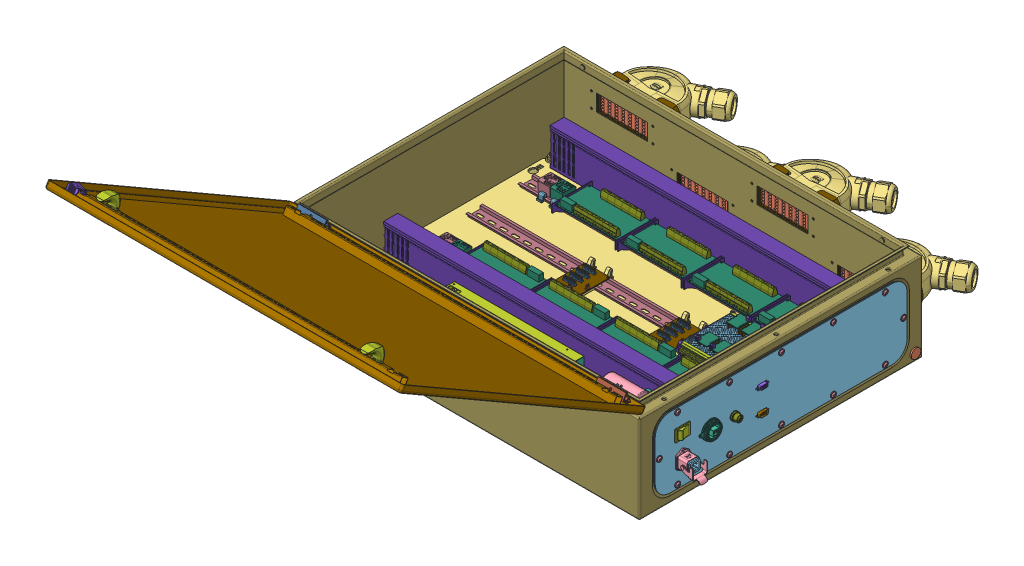
SolidWorks assembly _main_cabinet, configuration Default. Lengths in mm. (continued)
Components (placement in the parent): (continued)
- custom_perfboard-1: custom_perfboard [Default] at (151.5551 53.8 -20.003) size (162 55.7 125.4) (continued)
  - 3857 Adafruit Feather M4 Express headers 2-1: 3857 Adafruit Feather M4 Express headers 2 [Default] at (160.01 12.6 -94.45) x (-1 0 0) z (0 1 0) size (50.85 22.86 20.37) (continued)
    - 3857 Adafruit Feather M4 Express-1: 3857 Adafruit Feather M4 Express [Default] at origin size (50.85 22.86 6.37) (continued)
      - 3857 Adafruit Feather M4 Express(2)^3857 Adafruit Feather M4 Express-1: 3857 Adafruit Feather M4 Express(2)^3857 Adafruit Feather M4 Express [Default] at origin size (50.85 22.86 6.37) (virtual) (continued)
        - PCB Component^3857 Adafruit Feather M4 Express(2)_3857 Adafruit Feather M4 Express-1: PCB Component^3857 Adafruit Feather M4 Express(2)_3857 Adafruit Feather M4 Express [Default] at origin size (50.85 22.86 6.37) (virtual) (continued)
          - MBR120^PCB Component_3857 Adafruit Feather M4 Express(2)_3857 Adafruit Feather M4 Express-1: MBR120^PCB Component_3857 Adafruit Feather M4 Express(2)_3857 Adafruit Feather M4 Express [Default] at (10.35 12.319 1.57) x (-1 0 0) z (0 0 1) size (3.6 1.4 1.35) (virtual)
          - DMG341^PCB Component_3857 Adafruit Feather M4 Express(2)_3857 Adafruit Feather M4 Express-1: DMG341^PCB Component_3857 Adafruit Feather M4 Express(2)_3857 Adafruit Feather M4 Express [Default] at (9.398 9.842 1.57) size (3.04 2.64 1.12) (virtual)
          - 100K^PCB Component_3857 Adafruit Feather M4 Express(2)_3857 Adafruit Feather M4 Express-1: 100K^PCB Component_3857 Adafruit Feather M4 Express(2)_3857 Adafruit Feather M4 Express [Default] at (22.67 17.208 1.57) x (0 1 0) z (0 0 1) size (3.05 1.6 0.5) (virtual)
          - ATSAMD51J^PCB Component_3857 Adafruit Feather M4 Express(2)_3857 Adafruit Feather M4 Express-1: ATSAMD51J^PCB Component_3857 Adafruit Feather M4 Express(2)_3857 Adafruit Feather M4 Express [Default] at (30.162 11.049 1.57) x (0 1 0) z (0 0 1) size (9 9 0.8) (virtual)
          - 10uH^PCB Component_3857 Adafruit Feather M4 Express(2)_3857 Adafruit Feather M4 Express-1: 10uH^PCB Component_3857 Adafruit Feather M4 Express(2)_3857 Adafruit Feather M4 Express [Default] at (21.082 11.811 1.57) x (0 -1 0) z (0 0 1) size (2.7 2 2) (virtual)
    - header_m16-1: header_m16 [Default] at (5.08 1.27 -2.5) x (1 0 0) z (0 -1 0) size (40.64 11.5 2.5)
    - header_m12-1: header_m12 [Default] at (15.24 21.59 -2.5) x (1 0 0) z (0 -1 0) size (30.48 11.5 2.5)
    - header_f12-1: header_f12 [Default] at (15.115 21.59 -11) x (1 0 0) z (0 -1 0) size (30.73 11.5 2.5)
    - header_f16-1: header_f16 [Default] at (4.955 1.27 -11) x (1 0 0) z (0 -1 0) size (40.89 11.5 2.5)
  - dil_socket_2x7_populated-1: dil_socket_2x7_populated [Default] at (124.45 5.35 -38.57) x (0 0 -1) z (1 0 0) size (19.5 11.05 10.16)
    - dil_socket_2x7-1: dil_socket_2x7 [Default] at origin size (17.78 8.25 10.16)
    - dil_package_2x7-1: dil_package_2x7 [Default] at (-0.86 0.5 0) size (19.5 6.8 8.17)
  - header_m4-1: header_m4 [Default] at (8.88 4.1 -15.71) x (0 0 1) z (1 0 0) size (10.16 11.5 2.5)
  - header_m4-2: header_m4 [Default] at (6.34 4.1 -15.71) x (0 0 1) z (1 0 0) size (10.16 11.5 2.5)
  - screw_terminal_4x_2.54pitch_Multicomp_MP008515-1: screw_terminal_4x_2.54pitch_Multicomp_MP008515 [Default] at (153.05 1.6 -12.93) size (6.3 12.4 10.64)
  - screw_terminal_4x_2.54pitch_Multicomp_MP008515-2: screw_terminal_4x_2.54pitch_Multicomp_MP008515 [Default] at (153.05 1.6 -30.71) size (6.3 12.4 10.64)
  - 4-20mA_R_click_in_headers-6: 4-20mA_R_click_in_headers [Default] at (78.75 12.6 -33.49) x (-1 0 0) z (0 0 -1) size (25.4 24.5 30.48)
    - 4-20mA_R_click-1: 4-20mA_R_click [Default] at origin size (25.4 1.7 30.48)
    - header_m8-1: header_m8 [Default] at (1.25 -2.5 -22.86) x (0 0 1) z (-1 0 0) size (20.32 11.5 2.5)
    - header_m8-2: header_m8 [Default] at (24.15 -2.5 -2.54) x (0 0 -1) z (1 0 0) size (20.32 11.5 2.5)
    - screw_terminal_2x_2.54pitch-1: screw_terminal_2x_2.54pitch [Default] at (24.765 1.7 -23.545) x (0 0 -1) z (1 0 0) size (6.3 12.6 5.6)
    - header_f8-1: header_f8 [Default] at (24.15 -11 -2.415) x (0 0 -1) z (1 0 0) size (20.57 11.5 2.5)
    - header_f8-2: header_f8 [Default] at (1.25 -11 -22.985) x (0 0 1) z (-1 0 0) size (20.57 11.5 2.5)
  - Damen_CNC_2340-1_DIN-Rail_Mount_for_Eurocard_PCB_100x160mm_STEP214-1: Damen_CNC_2340-1_DIN-Rail_Mount_for_Eurocard_PCB_100x160mm_STEP214 [Default] at (158 -16.0731 10.0976) x (0 1 0) z (-1 0 0) size (37.6 125.4 162)
    - 2340-1_DIN-Rail_Mount_for_Eurocard_PCB_100x160mm_STEP214^Damen_CNC_2340-1_DIN-Rail_Mount_for_Eurocard_PCB_100x160mm_STEP214-1: 2340-1_DIN-Rail_Mount_for_Eurocard_PCB_100x160mm_STEP214^Damen_CNC_2340-1_DIN-Rail_Mount_for_Eurocard_PCB_100x160mm_STEP214 [Default] at origin size (37.6 125.4 162) (virtual)
      - eBom-prt0^2340-1_DIN-Rail_Mount_for_Eurocard_PCB_100x160mm_STEP214_Damen_CNC_2340-1_DIN-Rail_Mount_for_Eurocard_PCB_100x160mm_STEP214-1: eBom-prt0^2340-1_DIN-Rail_Mount_for_Eurocard_PCB_100x160mm_STEP214_Damen_CNC_2340-1_DIN-Rail_Mount_for_Eurocard_PCB_100x160mm_STEP214 [Default] at (-0.1593 -0.1673 0) size (21.5 122.6 156) (virtual)
      - eBom-prt1^2340-1_DIN-Rail_Mount_for_Eurocard_PCB_100x160mm_STEP214_Damen_CNC_2340-1_DIN-Rail_Mount_for_Eurocard_PCB_100x160mm_STEP214-1: eBom-prt1^2340-1_DIN-Rail_Mount_for_Eurocard_PCB_100x160mm_STEP214_Damen_CNC_2340-1_DIN-Rail_Mount_for_Eurocard_PCB_100x160mm_STEP214 [Default] at (-4.4655 32.2694 159) x (0 1 0) z (0 0 1) size (125.4 37.6 5) (virtual)
      - eBom-prt2^2340-1_DIN-Rail_Mount_for_Eurocard_PCB_100x160mm_STEP214_Damen_CNC_2340-1_DIN-Rail_Mount_for_Eurocard_PCB_100x160mm_STEP214-1: eBom-prt2^2340-1_DIN-Rail_Mount_for_Eurocard_PCB_100x160mm_STEP214_Damen_CNC_2340-1_DIN-Rail_Mount_for_Eurocard_PCB_100x160mm_STEP214 [Default] at (14.3514 121.3074 83.05) x (0.707107 -0.707107 0) z (0 0 1) size (5.4 5.4 15.85) (virtual)
      - eBom-prt2^2340-1_DIN-Rail_Mount_for_Eurocard_PCB_100x160mm_STEP214_Damen_CNC_2340-1_DIN-Rail_Mount_for_Eurocard_PCB_100x160mm_STEP214-2: eBom-prt2^2340-1_DIN-Rail_Mount_for_Eurocard_PCB_100x160mm_STEP214_Damen_CNC_2340-1_DIN-Rail_Mount_for_Eurocard_PCB_100x160mm_STEP214 [Default] at (9.3514 63.5574 83.05) x (0.707107 -0.707107 0) z (0 0 1) size (5.4 5.4 15.85) (virtual)
      - eBom-prt2^2340-1_DIN-Rail_Mount_for_Eurocard_PCB_100x160mm_STEP214_Damen_CNC_2340-1_DIN-Rail_Mount_for_Eurocard_PCB_100x160mm_STEP214-3: eBom-prt2^2340-1_DIN-Rail_Mount_for_Eurocard_PCB_100x160mm_STEP214_Damen_CNC_2340-1_DIN-Rail_Mount_for_Eurocard_PCB_100x160mm_STEP214 [Default] at (14.3514 5.8074 83.05) x (0.707107 -0.707107 0) z (0 0 1) size (5.4 5.4 15.85) (virtual)
      - eBom-prt3^2340-1_DIN-Rail_Mount_for_Eurocard_PCB_100x160mm_STEP214_Damen_CNC_2340-1_DIN-Rail_Mount_for_Eurocard_PCB_100x160mm_STEP214-1: eBom-prt3^2340-1_DIN-Rail_Mount_for_Eurocard_PCB_100x160mm_STEP214_Damen_CNC_2340-1_DIN-Rail_Mount_for_Eurocard_PCB_100x160mm_STEP214 [Default] at (-11.9191 -27.5171 -9.3242) x (0 1 0) z (0 0 -1) size (125.4 37.6 5) (virtual)
      - eBom-prt4^2340-1_DIN-Rail_Mount_for_Eurocard_PCB_100x160mm_STEP214_Damen_CNC_2340-1_DIN-Rail_Mount_for_Eurocard_PCB_100x160mm_STEP214-1: eBom-prt4^2340-1_DIN-Rail_Mount_for_Eurocard_PCB_100x160mm_STEP214_Damen_CNC_2340-1_DIN-Rail_Mount_for_Eurocard_PCB_100x160mm_STEP214 [Default] at (14.3514 114.3878 70.95) x (0.707107 0.707107 0) z (0 0 -1) size (5.15 5.15 16) (virtual)
      - eBom-prt4^2340-1_DIN-Rail_Mount_for_Eurocard_PCB_100x160mm_STEP214_Damen_CNC_2340-1_DIN-Rail_Mount_for_Eurocard_PCB_100x160mm_STEP214-2: eBom-prt4^2340-1_DIN-Rail_Mount_for_Eurocard_PCB_100x160mm_STEP214_Damen_CNC_2340-1_DIN-Rail_Mount_for_Eurocard_PCB_100x160mm_STEP214 [Default] at (-7.2051 63.5574 70.95) x (-0.707107 -0.707107 0) z (0 0 -1) size (5.15 5.15 16) (virtual)
      - eBom-prt4^2340-1_DIN-Rail_Mount_for_Eurocard_PCB_100x160mm_STEP214_Damen_CNC_2340-1_DIN-Rail_Mount_for_Eurocard_PCB_100x160mm_STEP214-3: eBom-prt4^2340-1_DIN-Rail_Mount_for_Eurocard_PCB_100x160mm_STEP214_Damen_CNC_2340-1_DIN-Rail_Mount_for_Eurocard_PCB_100x160mm_STEP214 [Default] at (-2.2051 5.8074 70.95) x (-0.707107 -0.707107 0) z (0 0 -1) size (5.15 5.15 16) (virtual)
- wpe_1_5_zz_-1016500000-1: wpe_1_5_zz_-1016500000 [Default] at (215.396 20.5 141.8) x (0 0 1) z (0 1 0) size (5.15 60 46.5)
- PTFIX_term_6-6X2,5 RD-1: PTFIX_term_6-6X2,5 RD [Default] at (-290.6026 29 -182.9) x (1 0 0) z (0 1 0) size (25.55 45.7 29.2)
  - 3273334-1: 3273334 [Default] at (12.775 14.3 0) x (1 0 0) z (0 -1 0) size (25.55 21.7 28.6)
    - 3273334_PTFIX_6_6x2.5_RD-select^3273334-1: 3273334_PTFIX_6_6x2.5_RD-select^3273334 [Default] at origin size (25.55 21.7 28.6) (virtual)
      - 3273334_PTFIX_6_6x2.5_RD-select^3273334_PTFIX_6_6x2.5_RD-select_3273334-1: 3273334_PTFIX_6_6x2.5_RD-select^3273334_PTFIX_6_6x2.5_RD-select_3273334 [Default] at (57.2719 -23.7678 -75.4575) x (0 0 1) z (-1 0 0) size (28.6 21.7 25.55) (virtual)
  - 3274056-1: 3274056 [Default] at (-5.15 -25.15 -7.5) size (10.3 45.7 11.95)
- PTFIX_term_6-6X2,5 BK-1: PTFIX_term_6-6X2,5 BK [Default] at (-264.6026 29 -182.9) x (1 0 0) z (0 1 0) size (25.56 45.7 29.2)
  - 3273344-1: 3273344 [Default] at (-12.775 -14.3 0) size (25.56 28.6 21.7)
    - 3273344_03_PTFIX-6-6X2-5-BK_3D^3273344-1: 3273344_03_PTFIX-6-6X2-5-BK_3D^3273344 [Default] at origin size (25.56 28.6 21.7) (virtual)
      - PTFIX_6_6X2.5_BK-select^3273344_03_PTFIX-6-6X2-5-BK_3D_3273344-1: PTFIX_6_6X2.5_BK-select^3273344_03_PTFIX-6-6X2-5-BK_3D_3273344 [Default] at (-57.2719 -75.4575 -23.7678) x (0 1 0) z (1 0 0) size (28.6 21.7 25.56) (virtual)
  - 3274056-1: 3274056 [Default] at (-5.15 -25.15 -7.5) size (10.3 45.7 11.95)
- PTFIX_term_6-6X2,5 BK-2: PTFIX_term_6-6X2,5 BK [Default] at (-264.6026 29 37.1) x (1 0 0) z (0 1 0) size (25.56 45.7 29.2)
  - 3273344-1: 3273344 [Default] at (-12.775 -14.3 0) size (25.56 28.6 21.7)
    - 3273344_03_PTFIX-6-6X2-5-BK_3D^3273344-1: 3273344_03_PTFIX-6-6X2-5-BK_3D^3273344 [Default] at origin size (25.56 28.6 21.7) (virtual)
      - PTFIX_6_6X2.5_BK-select^3273344_03_PTFIX-6-6X2-5-BK_3D_3273344-1: PTFIX_6_6X2.5_BK-select^3273344_03_PTFIX-6-6X2-5-BK_3D_3273344 [Default] at (-57.2719 -75.4575 -23.7678) x (0 1 0) z (1 0 0) size (28.6 21.7 25.56) (virtual)
  - 3274056-1: 3274056 [Default] at (-5.15 -25.15 -7.5) size (10.3 45.7 11.95)
- PTFIX_term_6-6X2,5 RD-3: PTFIX_term_6-6X2,5 RD [Default] at (-290.6026 29 37.1) x (1 0 0) z (0 1 0) size (25.55 45.7 29.2)
  - 3273334-1: 3273334 [Default] at (12.775 14.3 0) x (1 0 0) z (0 -1 0) size (25.55 21.7 28.6)
    - 3273334_PTFIX_6_6x2.5_RD-select^3273334-1: 3273334_PTFIX_6_6x2.5_RD-select^3273334 [Default] at origin size (25.55 21.7 28.6) (virtual)
      - 3273334_PTFIX_6_6x2.5_RD-select^3273334_PTFIX_6_6x2.5_RD-select_3273334-1: 3273334_PTFIX_6_6x2.5_RD-select^3273334_PTFIX_6_6x2.5_RD-select_3273334 [Default] at (57.2719 -23.7678 -75.4575) x (0 0 1) z (-1 0 0) size (28.6 21.7 25.55) (virtual)
  - 3274056-1: 3274056 [Default] at (-5.15 -25.15 -7.5) size (10.3 45.7 11.95)
- PTFIX_term_6-6X2,5 RD-4: PTFIX_term_6-6X2,5 RD [Default] at (244.6 29 261.225) x (0 0 -1) z (0 1 0) size (25.55 45.7 29.2)
  - 3273334-1: 3273334 [Default] at (12.775 14.3 0) x (1 0 0) z (0 -1 0) size (25.55 21.7 28.6)
    - 3273334_PTFIX_6_6x2.5_RD-select^3273334-1: 3273334_PTFIX_6_6x2.5_RD-select^3273334 [Default] at origin size (25.55 21.7 28.6) (virtual)
      - 3273334_PTFIX_6_6x2.5_RD-select^3273334_PTFIX_6_6x2.5_RD-select_3273334-1: 3273334_PTFIX_6_6x2.5_RD-select^3273334_PTFIX_6_6x2.5_RD-select_3273334 [Default] at (57.2719 -23.7678 -75.4575) x (0 0 1) z (-1 0 0) size (28.6 21.7 25.55) (virtual)
  - 3274056-1: 3274056 [Default] at (-5.15 -25.15 -7.5) size (10.3 45.7 11.95)
- PTFIX_term_6-6X2,5 RD-5: PTFIX_term_6-6X2,5 RD [Default] at (244.6 29 235.225) x (0 0 -1) z (0 1 0) size (25.55 45.7 29.2)
  - 3273334-1: 3273334 [Default] at (12.775 14.3 0) x (1 0 0) z (0 -1 0) size (25.55 21.7 28.6)
    - 3273334_PTFIX_6_6x2.5_RD-select^3273334-1: 3273334_PTFIX_6_6x2.5_RD-select^3273334 [Default] at origin size (25.55 21.7 28.6) (virtual)
      - 3273334_PTFIX_6_6x2.5_RD-select^3273334_PTFIX_6_6x2.5_RD-select_3273334-1: 3273334_PTFIX_6_6x2.5_RD-select^3273334_PTFIX_6_6x2.5_RD-select_3273334 [Default] at (57.2719 -23.7678 -75.4575) x (0 0 1) z (-1 0 0) size (28.6 21.7 25.55) (virtual)
  - 3274056-1: 3274056 [Default] at (-5.15 -25.15 -7.5) size (10.3 45.7 11.95)
- 1424137-1: 1424137 [Default] at (370.7479 93.5 100) x (0 0 -1) z (1 0 0) size (17.95 17.95 42.06)
- 8800_750_1_-1: 8800_750_1_ [Default] at (-340.9309 20 105.9684) x (1 0 0) z (0 -1 0) size (680 30 79.5)
- 8800_750_1_-2: 8800_750_1_ [Default] at (-340.9309 20 -246.5525) x (1 0 0) z (0 -1 0) size (680 30 79.5)
- Centipede_shield_v2_with_clips-1: Centipede_shield_v2_with_clips [Default] at (109.8725 32.8 -45.2) x (0 0 -1) z (1 0 0) size (87.91 21.69 53.5)
  - Centipede_shield_v2-1: Centipede_shield_v2 [Default] at origin size (73 1.6 53.5)
  - header_m2x10-1: header_m2x10 [Default] at (-15.25 4.1 6.25) x (0 0 -1) z (-1 0 0) size (25.4 11.5 5)
  - header_m2x10-2: header_m2x10 [Default] at (-1.25 4.1 6.25) x (0 0 -1) z (-1 0 0) size (25.4 11.5 5)
  - header_m2x10-3: header_m2x10 [Default] at (12.75 4.1 6.25) x (0 0 -1) z (-1 0 0) size (25.4 11.5 5)
  - header_m2x10-4: header_m2x10 [Default] at (26.75 4.1 6.25) x (0 0 -1) z (-1 0 0) size (25.4 11.5 5)
  - header_m3-1: header_m3 [Default] at (-25.75 4.1 7.75) x (0 0 -1) z (-1 0 0) size (7.62 11.5 2.5)
  - header_m3-2: header_m3 [Default] at (-5.28 4.1 23.96) x (-1 0 0) z (0 0 1) size (7.62 11.5 2.5)
  - header_m4-1: header_m4 [Default] at (-33.98 4.1 12.15) x (0 0 -1) z (-1 0 0) size (10.16 11.5 2.5)
  - DIN_rail_clip_73-1: DIN_rail_clip_73 [Default] at (39.6 -5.3 21.75) x (-1 0 0) z (0 0 -1) size (87.91 21.69 7.03)
  - DIN_rail_clip_73-2: DIN_rail_clip_73 [Default] at (39.6 -5.3 -14.75) x (-1 0 0) z (0 0 -1) size (87.91 21.69 7.03)
- Centipede_shield_v2_with_clips-2: Centipede_shield_v2_with_clips [Default] at (-90.1275 32.8 -45.2) x (0 0 -1) z (1 0 0) size (87.91 21.69 53.5)
  - Centipede_shield_v2-1: Centipede_shield_v2 [Default] at origin size (73 1.6 53.5)
  - header_m2x10-1: header_m2x10 [Default] at (-15.25 4.1 6.25) x (0 0 -1) z (-1 0 0) size (25.4 11.5 5)
  - header_m2x10-2: header_m2x10 [Default] at (-1.25 4.1 6.25) x (0 0 -1) z (-1 0 0) size (25.4 11.5 5)
  - header_m2x10-3: header_m2x10 [Default] at (12.75 4.1 6.25) x (0 0 -1) z (-1 0 0) size (25.4 11.5 5)
  - header_m2x10-4: header_m2x10 [Default] at (26.75 4.1 6.25) x (0 0 -1) z (-1 0 0) size (25.4 11.5 5)
  - header_m3-1: header_m3 [Default] at (-25.75 4.1 7.75) x (0 0 -1) z (-1 0 0) size (7.62 11.5 2.5)
  - header_m3-2: header_m3 [Default] at (-5.28 4.1 23.96) x (-1 0 0) z (0 0 1) size (7.62 11.5 2.5)
  - header_m4-1: header_m4 [Default] at (-33.98 4.1 12.15) x (0 0 -1) z (-1 0 0) size (10.16 11.5 2.5)
  - DIN_rail_clip_73-1: DIN_rail_clip_73 [Default] at (39.6 -5.3 21.75) x (-1 0 0) z (0 0 -1) size (87.91 21.69 7.03)
  - DIN_rail_clip_73-2: DIN_rail_clip_73 [Default] at (39.6 -5.3 -14.75) x (-1 0 0) z (0 0 -1) size (87.91 21.69 7.03)
- 09200030301_assy-1: 09200030301_assy [Default] at (380.5 68.5 210) x (0 0 1) z (0 1 0) size (33.6 46.56 42.89)
  - 09200030301-1: 09200030301 [Default] at origin size (33.6 46.56 42.89)
  - 09200032611-1: 09200032611 [Default] at origin size (23.4 27.1 23.7)
- wpe_1_5_zz_-1016500000-2: wpe_1_5_zz_-1016500000 [Default] at (215.396 20.5 136.8) x (0 0 1) z (0 1 0) size (5.15 60 46.5)
- wpe_1_5_zz_-1016500000-3: wpe_1_5_zz_-1016500000 [Default] at (215.396 20.5 131.8) x (0 0 1) z (0 1 0) size (5.15 60 46.5)
- wpe_1_5_zz_-1016500000-4: wpe_1_5_zz_-1016500000 [Default] at (215.396 20.5 126.8) x (0 0 1) z (0 1 0) size (5.15 60 46.5)
- px0844-b-0m50-b.stp-1: px0844-b-0m50-b.stp [Default] at (388.965 93.5 150) x (-1 0 0) z (0 0 -1) size (147.68 37.95 45.1)
- c1350al.stp-1: c1350al.stp [Default] at (382.53 118.5 210) x (0 0 1) z (-1 0 0) size (32.24 24.9 33.57)
- db9_panel_mount_IP67_female-1: db9_panel_mount_IP67_female [Default] at (379 118.5 40) x (0 0 -1) z (1 0 0) size (39.4 21 14.45)
- db9_panel_mount_IP67_male-1: db9_panel_mount_IP67_male [Default] at (379 68.5 40) x (0 0 -1) z (1 0 0) size (39.4 21 14.45)
Mates (geometry in assembly coordinates):
- Coincident3: coincident aligned: plane of DIN_rail_35x7.5_long-2 through (340 20 -180) normal (0 -1 0); plane of DIN_rail_35x7.5_long-1 through (340 20 -70) normal (0 -1 0)
- Coincident4: coincident aligned: plane of DIN_rail_35x7.5_long-1 through (340 20 -70) normal (0 -1 0); plane of DIN_rail_35x7.5_long-3 through (340 20 40) normal (0 -1 0)
- Coincident6: coincident aligned: plane of DIN_rail_35x7.5_long-1 through (-340 20 -70) normal (1 0 0); plane of DIN_rail_35x7.5_long-2 through (-340 20 -180) normal (1 0 0)
- Coincident7: coincident aligned: plane of DIN_rail_35x7.5_long-1 through (-340 20 -70) normal (1 0 0); plane of DIN_rail_35x7.5_long-3 through (-340 20 40) normal (1 0 0)
- Coincident18: coincident anti-aligned: plane of DIN_rail_35x7.5_long-3 through (340 27.5 22.5) normal (0 1 0); plane of Sanwo_16ch_mosfet_board-2/Sanwo_16ch_mosfet_board_DIN_rail_support-2 through (-242.3811 27.5 22.5) normal (0 -1 0)
- Coincident19: coincident anti-aligned: plane of DIN_rail_35x7.5_long-3 through (340 26.5 22.5) normal (0 0 -1); plane of Sanwo_16ch_mosfet_board-2/Sanwo_16ch_mosfet_board_DIN_rail_support-2 through (-242.3811 26 22.5) normal (0 0 1)
- Coincident22: coincident aligned: plane of Harting Mod.24-HSE-M40-2/19410240301_100198179MOD000C-HOUSING-1 through (479.2399 -47.9361 -217.1325) normal (-0.008727 0 0.999962); plane of Harting Mod.24-HSE-M40-4/19410240301_100198179MOD000C-HOUSING-1 through (480.3409 -47.9362 -217.1229) normal (-0.008727 0 0.999962)
- Parallel5: parallel aligned: plane of Harting Mod.24-HSE-M40-1 through (-255 123.75 -322) normal (0 1 0)
- Coincident23: coincident anti-aligned: plane of DIN_rail_35x7.5_long-2 through (340 27.5 -197.5) normal (0 1 0); plane of Sanwo_16ch_mosfet_board-1/Sanwo_16ch_mosfet_board_DIN_rail_support-2 through (-108.8811 27.5 -162.5) normal (0 -1 0)
- Distance6: distance = 110 mm aligned: plane of DIN_rail_35x7.5_long-1 through (-340 20 -70) normal (0 0 -1); plane of DIN_rail_35x7.5_long-2 through (-340 20 -180) normal (0 0 -1)
- Distance7: distance = 110 mm aligned: plane of DIN_rail_35x7.5_long-1 through (-340 20 -70) normal (0 0 -1); plane of DIN_rail_35x7.5_long-3 through (-340 20 40) normal (0 0 -1)
- Coincident31: coincident anti-aligned: plane of DNR30_60-1 through (265.81 27.5 221.45) normal (0 -1 0); plane of DIN_rail_35x7.5_psus-1 through (265 27.5 275) normal (0 1 0)
- Coincident32: coincident anti-aligned: plane of DNR30_60-1 through (230 27.5 221.45) normal (1 0 0); plane of DIN_rail_35x7.5_psus-1 through (230 26.5 275) normal (-1 0 0)
- Coincident33: coincident anti-aligned: plane of CUI_PSK-10D-3-DIN-1 through (249 27.5 163.7) normal (0 -1 0); plane of DIN_rail_35x7.5_psus-1 through (230 27.5 275) normal (0 1 0)
- Coincident34: coincident anti-aligned: plane of CUI_PSK-10D-3-DIN-1 through (230 27.25 175.1) normal (1 0 0); plane of DIN_rail_35x7.5_psus-1 through (230 26.5 275) normal (-1 0 0)
- Coincident36: coincident anti-aligned: plane of DIN_rail_35x7.5_psus-1 through (230 27.5 275) normal (0 1 0); plane of wpe_1_5_zz_-1016500000-1 through (230 27.5 144.38) normal (0 -1 0)
- Coincident37: coincident anti-aligned: plane of DIN_rail_35x7.5_psus-1 through (230 26.5 275) normal (-1 0 0); plane of wpe_1_5_zz_-1016500000-1 through (230 25.546 144.375) normal (1 0 0)
- Coincident38: coincident aligned: plane of DIN_rail_35x7.5_long-2 through (-340 20 -180) normal (0 0 -1); plane of PTFIX_term_6-6X2,5 RD-1 through (-290.6026 29 -180) normal (0 0 -1)
- Coincident42: coincident aligned: plane of DIN_rail_35x7.5_long-2 through (340 27.5 -162.5) normal (0 1 0); plane of PTFIX_term_6-6X2,5 RD-1 through (-290.6026 27.5 -182.9) normal (0 1 0)
- Parallel7: parallel anti-aligned: plane of txln750_3D_drawing.stp-1 through (-34.7816 83.2954 180) normal (0 0 -1)
- Coincident47: coincident aligned: plane of DIN_rail_35x7.5_long-2 through (340 27.5 -162.5) normal (0 1 0); plane of PTFIX_term_6-6X2,5 BK-1 through (-264.6026 27.5 -182.9) normal (0 1 0)
- Coincident55: coincident aligned: plane of DIN_rail_35x7.5_psus-1 through (265 27.5 275) normal (0 1 0); plane of PTFIX_term_6-6X2,5 RD-4 through (244.6 27.5 261.225) normal (0 1 0)
- Coincident56: coincident anti-aligned: plane of DIN_rail_35x7.5_psus-1 through (247.5 20 125) normal (1 0 0); plane of PTFIX_term_6-6X2,5 RD-4 through (247.5 29 261.225) normal (-1 0 0)
- Coincident57: coincident aligned: plane of DIN_rail_35x7.5_psus-1 through (265 27.5 275) normal (0 1 0); plane of PTFIX_term_6-6X2,5 RD-5 through (244.6 27.5 235.225) normal (0 1 0)
- Coincident58: coincident aligned: plane of PTFIX_term_6-6X2,5 RD-4 through (244.6 29 261.225) normal (-1 0 0); plane of PTFIX_term_6-6X2,5 RD-5 through (244.6 29 235.225) normal (-1 0 0)
- Distance14: distance = 26 mm aligned: plane of PTFIX_term_6-6X2,5 RD-5 through (244.6 29 235.225) normal (0 0 -1); plane of PTFIX_term_6-6X2,5 RD-4 through (244.6 29 261.225) normal (0 0 -1)
- Coincident61: coincident aligned: plane of 1076_000_1_customized-1 through (0 0 0) normal (0 1 0)
- Coincident62: coincident anti-aligned: plane of 1076_000_1_customized-1 through (0 0 0) normal (0 0 -1)
- Coincident63: coincident anti-aligned: plane of assembly through (0 0 0) normal (1 0 0); plane of 1076_000_1_customized-1 through (0 0 0) normal (-1 0 0)
- Distance5: distance = 22 mm aligned: plane of Harting Mod.24-HSE-M40-1 through (-255 123.75 -322) normal (0 0 -1); plane of 1076_000_1_customized-1/1076_000_1__41_customized-1 through (-380 187.5 -300) normal (0 0 -1)
- Coincident65: coincident anti-aligned: plane of 1076_000_1_-1/1076_000_1__10-1 through (344.5 20 274.0774) normal (0 1 0); plane of DIN_rail_35x7.5_long-1 through (340 20 -70) normal (0 -1 0)
- Distance15: distance = 70 mm anti-aligned: plane of DIN_rail_35x7.5_long-1 through (-340 20 -70) normal (0 0 -1)
- Coincident69: coincident anti-aligned: plane of 1076_000_1_customized-1 through (0 0 0) normal (-1 0 0); plane of DIN_rail_35x7.5_long-1 through (0 20 -70) normal (1 0 0)
- Coincident70: coincident anti-aligned: plane of 1076_000_1_-1/1076_000_1__10-1 through (344.5 20 274.0774) normal (0 1 0); plane of DIN_rail_35x7.5_psus-1 through (247.5 20 275) normal (0 -1 0)
- Distance16: distance = 120 mm aligned: plane of 1076_000_1_-1/1076_000_1__10-1 through (367.5 17.5 243) normal (1 0 0); plane of DIN_rail_35x7.5_psus-1 through (247.5 20 125) normal (1 0 0)
- Coincident74: coincident aligned: plane of 1076_000_1_-1/1076_000_1__10-1 through (-343.5 17.5 275) normal (0 0 1); plane of DIN_rail_35x7.5_psus-1 through (247.5 20 275) normal (0 0 1)
- Coincident75: coincident anti-aligned: plane of 1076_000_1_-1/1076_000_1__10-1 through (344.5 20 274.0774) normal (0 1 0); plane of txln750_3D_drawing.stp-1/CASE.stp-1 through (-171.8816 20 140.0168) normal (0 -1 0)
- Distance17: distance = 180 mm aligned: plane of txln750_3D_drawing.stp-1 through (-34.7816 83.2954 180) normal (0 0 -1); plane of 1076_000_1_customized-1 through (0 0 0) normal (0 0 -1)
- Coincident79: coincident anti-aligned: plane of 1076_000_1_customized-1/1076_000_1__25_customized-1 through (380.5 136 235) normal (1 0 0); circle of 1424137-1
- Coincident80: coincident aligned: plane of 1076_000_1_customized-1/1076_000_1__25_customized-1 through (380.5 93.5 0) normal (0 1 0); plane of 1424137-1 through (370.7479 93.5 100) normal (0 1 0)
- Coincident81: coincident anti-aligned: plane of 1076_000_1_-1/1076_000_1__10-1 through (344.5 20 274.0774) normal (0 1 0); plane of 8800_750_1_-1 through (1659.0691 20 118.3684) normal (0 -1 0)
- Coincident82: coincident anti-aligned: plane of 1076_000_1_-1/1076_000_1__10-1 through (344.5 20 274.0774) normal (0 1 0); plane of 8800_750_1_-2 through (1659.0691 20 -234.1525) normal (0 -1 0)
- Coincident83: coincident aligned: plane of 8800_750_1_-1 through (-340.9309 20 105.9684) normal (1 0 0); plane of 8800_750_1_-2 through (-340.9309 20 -246.5525) normal (1 0 0)
- Coincident84: coincident aligned: plane of Sanwo_16ch_mosfet_board-1/Sanwo_16ch_mosfet_board_DIN_rail_support-1 through (-243.8811 27.5 -180) normal (-1 0 0); plane of Sanwo_16ch_mosfet_board-2/Sanwo_16ch_mosfet_board_DIN_rail_support-2 through (-243.8811 27.5 40) normal (-1 0 0)
- Coincident85: coincident anti-aligned: plane of DIN_rail_35x7.5_long-2 through (340 26.5 -197.5) normal (0 0 -1); plane of Sanwo_16ch_mosfet_board-1/Sanwo_16ch_mosfet_board_DIN_rail_support-1 through (-243.8811 27.5 -197.5) normal (0 0 1)
- Coincident89: coincident aligned: plane of Harting Mod.24-HSE-M40-1 through (-255 123.75 -322) normal (0 0 -1); plane of Harting Mod.24-HSE-M40-12 through (-85.3206 69.3824 -322) normal (0 0 -1)
- Concentric3: concentric aligned: circle of 1076_000_1_customized-1/1076_000_1__41_customized-1; circle of Harting Mod.24-HSE-M40-1/19410240301_100198179MOD000C-HOUSING-1
- Coincident91: coincident aligned: plane of Harting Mod.24-HSE-M40-1 through (-255 123.75 -322) normal (0 0 -1); plane of Harting Mod.24-HSE-M40-14 through (-85 63.75 -322) normal (0 0 -1)
- Coincident92: coincident aligned: plane of Harting Mod.24-HSE-M40-1 through (-255 123.75 -322) normal (0 0 -1); plane of Harting Mod.24-HSE-M40-15 through (85 123.75 -322) normal (0 0 -1)
- Coincident93: coincident aligned: plane of Harting Mod.24-HSE-M40-1 through (-255 123.75 -322) normal (0 0 -1); plane of Harting Mod.24-HSE-M40-16 through (255 63.75 -322) normal (0 0 -1)
- Parallel11: parallel aligned: plane of Harting Mod.24-HSE-M40-14 through (-85 63.75 -322) normal (0 1 0)
- Parallel12: parallel aligned: plane of Harting Mod.24-HSE-M40-15 through (85 123.75 -322) normal (0 1 0)
- Parallel13: parallel aligned: plane of Harting Mod.24-HSE-M40-16 through (255 63.75 -322) normal (0 1 0)
- Concentric4: concentric anti-aligned: circle of 1076_000_1_customized-1/1076_000_1__41_customized-1; circle of Harting Mod.24-HSE-M40-14/19410240301_100198179MOD000C-HOUSING-1
- Concentric5: concentric anti-aligned: circle of 1076_000_1_customized-1/1076_000_1__41_customized-1; circle of Harting Mod.24-HSE-M40-15/19410240301_100198179MOD000C-HOUSING-1
- Concentric6: concentric anti-aligned: circle of 1076_000_1_customized-1/1076_000_1__41_customized-1; circle of Harting Mod.24-HSE-M40-16/19410240301_100198179MOD000C-HOUSING-1
- Coincident94: coincident aligned: plane of PTFIX_term_6-6X2,5 RD-1 through (-290.6026 29 -182.9) normal (0 0 -1); plane of PTFIX_term_6-6X2,5 BK-1 through (-264.6026 29 -182.9) normal (0 0 -1)
- Distance19: distance = 26 mm aligned: plane of PTFIX_term_6-6X2,5 RD-1 through (-290.6026 29 -182.9) normal (1 0 0); plane of PTFIX_term_6-6X2,5 BK-1 through (-264.6026 29 -182.9) normal (1 0 0)
- Coincident95: coincident aligned: plane of DIN_rail_35x7.5_long-1 through (-340 20 -70) normal (0 0 -1); plane of custom_perfboard-1/Damen_CNC_2340-1_DIN-Rail_Mount_for_Eurocard_PCB_100x160mm_STEP214-1 through (309.5551 37.7269 -70) normal (0 0 -1)
- Coincident96: coincident anti-aligned: plane of DIN_rail_35x7.5_long-1 through (340 27.5 -52.5) normal (0 1 0); plane of custom_perfboard-1/Damen_CNC_2340-1_DIN-Rail_Mount_for_Eurocard_PCB_100x160mm_STEP214-1/2340-1_DIN-Rail_Mount_for_Eurocard_PCB_100x160mm_STEP214^Damen_CNC_2340-1_DIN-Rail_Mount_for_Eurocard_PCB_100x160mm_STEP214-1/eBom-prt1^2340-1_DIN-Rail_Mount_for_Eurocard_PCB_100x160mm_STEP214_Damen_CNC_2340-1_DIN-Rail_Mount_for_Eurocard_PCB_100x160mm_STEP214-1 through (160.3853 27.5 -52.503) normal (0 -1 0)
- Coincident98: coincident aligned: plane of 1076_000_1_customized-1/1076_000_1__25_customized-1 through (380.5 136 235) normal (1 0 0); plane of 09200030301_assy-1 through (380.5 68.5 210) normal (1 0 0)
- Coincident101: coincident aligned: plane of 1076_000_1_customized-1/1076_000_1__25_customized-1 through (380.5 68.5 0) normal (0 1 0); plane of 09200030301_assy-1 through (380.5 68.5 210) normal (0 1 0)
- Distance20: distance = 1 mm aligned: plane of DIN_rail_35x7.5_psus-1 through (247.5 20 275) normal (0 0 1); plane of PTFIX_term_6-6X2,5 RD-4/3273334-1/3273334_PTFIX_6_6x2.5_RD-select.stp-1/3273334_PTFIX_6_6x2.5_RD-select.stp-1 through (230.8 38.7385 274) normal (0 0 1)
- Distance26: distance = 1 mm anti-aligned: plane of DNR30_60-1 through (253.3345 -2.4064 221.45) normal (0 0 1); plane of PTFIX_term_6-6X2,5 RD-5/3273334-1/3273334_PTFIX_6_6x2.5_RD-select.stp-1/3273334_PTFIX_6_6x2.5_RD-select.stp-1 through (239.45 50.6 222.45) normal (0 0 -1)
- Distance27: distance = 1 mm anti-aligned: plane of CUI_PSK-10D-3-DIN-1 through (249 28 179.45) normal (0 0 1); plane of DNR30_60-1 through (253.3345 -2.4064 180.45) normal (0 0 -1)
- Distance28: distance = 1 mm anti-aligned: plane of CUI_PSK-10D-3-DIN-1 through (249 28 147.95) normal (0 0 -1); plane of wpe_1_5_zz_-1016500000-1 through (263.5474 66.2427 146.95) normal (0 0 1)
- Coincident111: coincident anti-aligned: plane of 1076_000_1_customized-1/1076_000_1__25_customized-1 through (380.5 93.5 210) normal (0 0 -1); plane of 09200030301_assy-1 through (380.5 68.5 210) normal (0 0 1)
- Coincident112: coincident aligned: plane of 1076_000_1_customized-1/1076_000_1__25_customized-1 through (380.5 93.5 150) normal (0 0 -1); plane of px0844-b-0m50-b.stp-1 through (388.965 93.5 150) normal (0 0 -1)
- Coincident113: coincident anti-aligned: plane of 1076_000_1_customized-1/1076_000_1__25_customized-1 through (380.5 136 235) normal (1 0 0); plane of px0844-b-0m50-b.stp-1 through (380.5 93.5 150) normal (-1 0 0)
- Concentric7: concentric anti-aligned: cylinder of 1076_000_1_customized-1/1076_000_1__25_customized-1 through (379 93.5 150) axis (1 0 0) radius 13.75; cylinder of px0844-b-0m50-b.stp-1 through (383.6269 93.5 150) axis (-1 0 0) radius 8.7266
- Coincident114: coincident anti-aligned: plane of 1076_000_1_customized-1/1076_000_1__25_customized-1 through (380.5 136 235) normal (1 0 0); plane of c1350al.stp-1 through (380.5 118.5 210) normal (-1 0 0)
- Coincident115: coincident anti-aligned: plane of 1076_000_1_customized-1/1076_000_1__25_customized-1 through (380.5 93.5 210) normal (0 0 -1); plane of c1350al.stp-1 through (382.53 118.5 210) normal (0 0 1)
- Coincident116: coincident aligned: plane of 1076_000_1_customized-1/1076_000_1__25_customized-1 through (380.5 118.5 0) normal (0 1 0); plane of c1350al.stp-1 through (382.53 118.5 210) normal (0 1 0)
- Concentric8: concentric anti-aligned: cylinder of 1076_000_1_customized-1/1076_000_1__25_customized-1 through (379 93.5 100) axis (1 0 0) radius 8.25; cylinder of 1424137-1 through (394.4779 93.5 100) axis (-1 0 0) radius 8
- Coincident117: coincident anti-aligned: plane of DIN_rail_35x7.5_long-1 through (340 27.5 -87.5) normal (0 1 0); plane of Centipede_shield_v2_with_clips-1/DIN_rail_clip_73-1 through (124.6225 27.5 -85.9769) normal (0 -1 0)
- Coincident118: coincident anti-aligned: plane of DIN_rail_35x7.5_long-1 through (340 26.5 -87.5) normal (0 0 -1); plane of Centipede_shield_v2_with_clips-1/DIN_rail_clip_73-1 through (124.6225 26.2 -87.5) normal (0 0 1)
- Coincident119: coincident: plane of 1076_000_1_customized-1/1076_000_1__25_customized-1 through (379 136 235) normal (-1 0 0); plane of db9_panel_mount_IP67_female-1 through (379 124.9064 40) normal (1 0 0)
- Coincident120: coincident: plane of 1076_000_1_customized-1/1076_000_1__25_customized-1 through (379 136 235) normal (-1 0 0); plane of db9_panel_mount_IP67_male-1 through (379 48.8873 40) normal (1 0 0)
- Coincident121: coincident: plane of 1076_000_1_customized-1/1076_000_1__25_customized-1 through (380.5 93.5 40) normal (0 0 -1); plane of db9_panel_mount_IP67_female-1 through (379 124.9064 40) normal (0 0 -1)
- Coincident122: coincident: plane of 1076_000_1_customized-1/1076_000_1__25_customized-1 through (380.5 93.5 40) normal (0 0 -1); plane of db9_panel_mount_IP67_male-1 through (379 48.8873 40) normal (0 0 -1)
- Coincident123: coincident aligned: plane of 1076_000_1_customized-1/1076_000_1__25_customized-1 through (380.5 118.5 0) normal (0 1 0); plane of db9_panel_mount_IP67_female-1 through (379 118.5 40) normal (0 1 0)
- Coincident124: coincident aligned: plane of 1076_000_1_customized-1/1076_000_1__25_customized-1 through (380.5 68.5 0) normal (0 1 0); plane of db9_panel_mount_IP67_male-1 through (379 68.5 40) normal (0 1 0)
